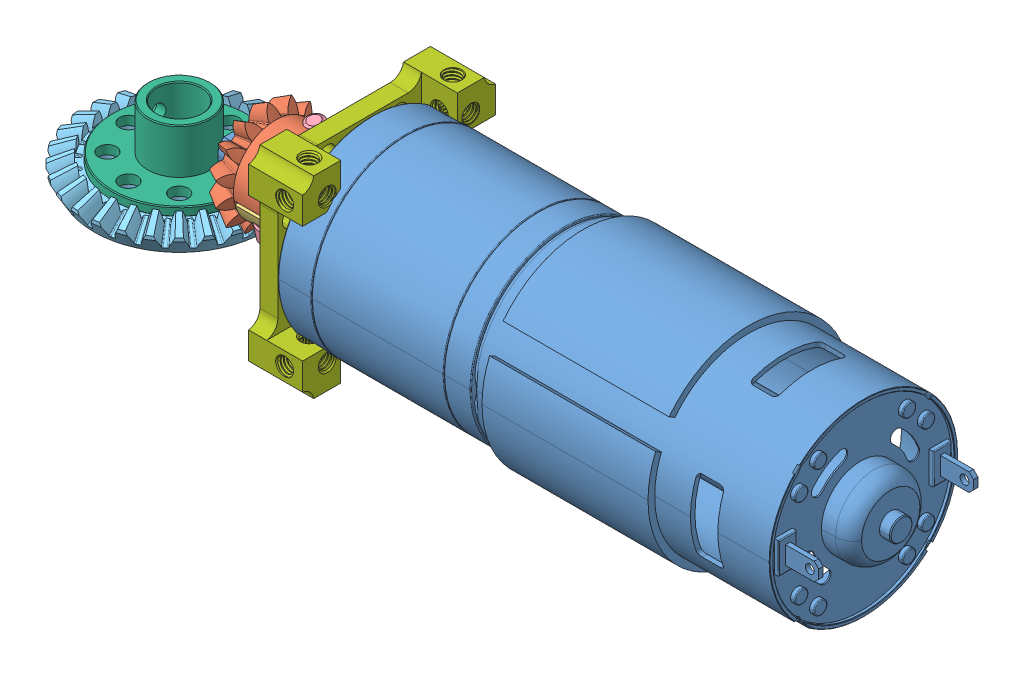
SolidWorks assembly 皮带电机装配体, configuration 默认. Lengths in mm.
Overall size (182.3 67.11 64.42).
10 component instances, 7 part files, 8 mates.
Components (placement in the parent):
- 发射轮电机1-1: 发射轮电机1 [默认] at (-31.948 68.6302 -206.7966) size (148.5 67.11 64.42)
- 3204-0002-0002 assembly-1: 3204-0002-0002 assembly [默认] at (-82.9257 129.4143 -179.1986) x (0 1 0) z (0 0 1) size (28.67 52.38 42.6)
  - 2306-4008-0014 assembly(2)-1: 2306-4008-0014 assembly(2) [默认] at (-86.5036 -22.1715 14.0673) x (0 1 0) z (-0.223733 0 0.97465) size (15.4 23.81 24.42)
    - 2306-4008-0014-1: 2306-4008-0014 [默认] at (-4.2928 -28.4802 22.5212) size (15.32 23.81 24.42)
    - 2306-4008-0014 clamp-1: 2306-4008-0014 clamp [默认] at (-4.2932 -28.4802 22.5212) size (9.55 8.86 18.72)
    - 2800-0004-0012_90128A207-1: 2800-0004-0012_90128A207 [默认] at (-8.9015 -37.2302 16.6212) x (0.549526 0 0.835476) z (0 -1 0) size (7 7 16.17)
    - 2800-0004-0012_90128A207-2: 2800-0004-0012_90128A207 [默认] at (-8.9015 -37.2302 28.4212) x (0.549526 0 -0.835476) z (0 -1 0) size (7 7 16.17)
  - 2307-0014-0028-1: 2307-0014-0028 [默认] at (-76.6728 -4.8452 42.3896) size (6.41 42.6 42.6)
- 齿轮组法兰-1: 齿轮组法兰 [默认] at (-78.0805 56.1302 -136.809) x (0 1 0) z (0 0 1) size (12 30 30) (hidden)
- 电机转向座1-1: 电机转向座1 [默认] at (-41.0801 65.9902 -136.809) x (0 0 -1) z (0 -1 0) size (43.24 12.23 43.24)
Mates (geometry in assembly coordinates):
- 同心9: concentric: circle of 发射轮电机1-1; circle of 电机转向座1-1
- 重合8: coincident: plane of 发射轮电机1-1 through (-37.0801 65.6302 -136.809) normal (-1 0 0); plane of 电机转向座1-1 through (-67.0487 65.9902 -137.7099) normal (1 0 0)
- 重合1: coincident anti-aligned: plane of 3204-0002-0002 assembly-1/2307-0014-0028-1 through (-78.0805 56.1302 -136.809) normal (0 1 0); plane of 齿轮组法兰-1 through (-78.0805 56.1302 -136.809) normal (0 -1 0)
- 同心1: concentric aligned: cylinder of 3204-0002-0002 assembly-1/2307-0014-0028-1 through (-78.0805 52.1302 -136.809) axis (0 1 0) radius 7; cylinder of 齿轮组法兰-1 through (-78.0805 56.1302 -136.809) axis (0 1 0) radius 5
- 同心2: concentric aligned: cylinder of 3204-0002-0002 assembly-1/2307-0014-0028-1 through (-89.3942 52.1302 -136.809) axis (0 1 0) radius 2; cylinder of 齿轮组法兰-1 through (-89.3942 56.1302 -136.809) axis (0 1 0) radius 2
- 同心10: concentric: circle of 发射轮电机1-1; circle of 3204-0002-0002 assembly-1/2306-4008-0014 assembly(2)-1/2306-4008-0014 clamp-1
- 距离2: distance = 10 mm: plane of 3204-0002-0002 assembly-1/2306-4008-0014 assembly(2)-1/2306-4008-0014 clamp-1 through (-47.0801 65.6302 -136.809) normal (1 0 0); plane of 发射轮电机1-1 through (-37.0801 65.6302 -136.809) normal (-1 0 0)
- 平行2: parallel aligned: plane of 3204-0002-0002 assembly-1/2307-0014-0028-1 through (-78.0805 54.1302 -136.809) normal (0 -1 0); plane of 电机转向座1-1 through (-37.0801 46.9902 -136.809) normal (0 -1 0)
